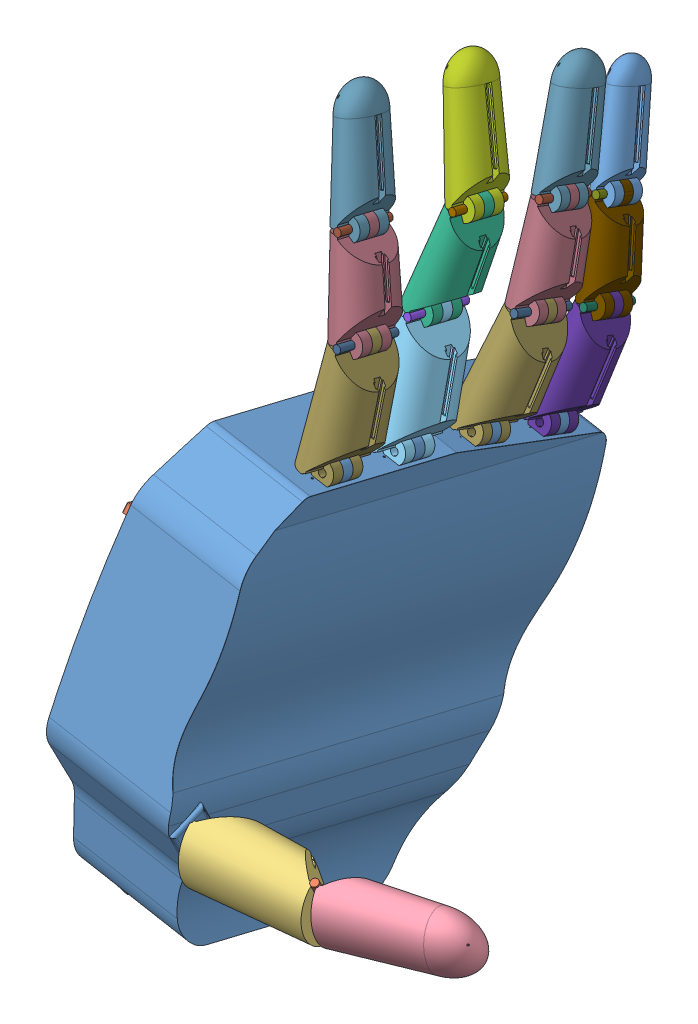
SolidWorks assembly hand_ass_v2, configuration Default. Lengths in mm.
Overall size (122.49 222.13 158.08).
29 component instances, 20 part files, 48 mates.
Components (placement in the parent):
- mainbody_v2-4: mainbody_v2 [Default] at (1393.0939 256.2845 230.0733) x (-0.03967 -0.262646 -0.964076) z (0.98509 -0.171926 0.006304) size (116.82 115 48.77)
- Mate1t-4: Mate1t [Default] at (1443.7902 225.3063 267.9284) x (0.146425 0.857082 0.493933) z (0.670742 0.280983 -0.686407) size (23 2 2)
- Part1t-3: Part1t [Default] at (1431.2867 235.9478 276.4521) x (0.146425 0.857082 0.493933) z (-0.086451 0.508491 -0.856716) size (80.14 37 28.83)
- Part2t-3: Part2t [Default] at (1462.1105 235.1801 268.6506) x (0.146425 0.857082 0.493933) z (-0.264208 0.51506 -0.815419) size (22.13 38.57 15.06)
- Part1m-2: Part1m [Default] at (1414.4402 322.5973 216.192) x (-0.03967 -0.262646 -0.964076) z (0.999177 -0.002227 -0.040508) size (67.14 37 33.3)
- Part2m-2: Part2m [Default] at (1416.9612 349.6562 208.7166) x (-0.03967 -0.262646 -0.964076) z (0.980971 -0.193758 0.012421) size (18.99 32 13.25)
- Part3m-2: Part3m [Default] at (1414.6092 375.7736 201.6979) x (-0.03967 -0.262646 -0.964076) z (0.948609 0.293255 -0.118926) size (16.1 35.5 11.04)
- Mate1-2: Mate1 [Default] at (1415.2589 339.0559 221.0098) x (-0.03967 -0.262646 -0.964076) z (0.870094 0.465305 -0.162567) size (18 2 2)
- Mate2-2: Mate2 [Default] at (1420.1608 363.3694 213.1471) x (-0.03967 -0.262646 -0.964076) z (0.88018 0.447523 -0.158138) size (16 2 2)
- Mate1i-7: Mate1i [Default] at (1419.1567 328.7029 194.6213) x (-0.061096 -0.383846 -0.921374) z (0.853883 0.457912 -0.247388) size (18 2 2)
- Mate2i-7: Mate2i [Default] at (1415.3779 344.2512 169.9444) x (0.061096 0.383846 0.921374) z (-0.994886 0.097798 0.025228) size (16 2 2)
- Part1i-6: Part1i [Default] at (1415.7923 312.9467 191.6404) x (-0.061096 -0.383846 -0.921374) z (0.98509 -0.171926 0.006304) size (67.02 35 36.64)
- Part2-6: Part2 [Default] at (1416.6054 336.7334 181.6776) x (-0.061096 -0.383846 -0.921374) z (0.991581 0.082247 -0.100016) size (18.98 30 13.22)
- Part3i-6: Part3i [Default] at (1412.8163 360.7728 171.9137) x (-0.061096 -0.383846 -0.921374) z (0.980311 0.150581 -0.127736) size (16.1 33.51 11.04)
- Mate1p-2: Mate1p [Default] at (1417.5601 318.7755 173.3582) x (-0.061096 -0.383846 -0.921374) z (0.991721 -0.127797 -0.01252) size (16 2 2)
- Mate2p-2: Mate2p [Default] at (1411.96 339.126 164.166) x (-0.061096 -0.383846 -0.921374) z (0.997555 0.007899 -0.069439) size (14 2 2)
- Part1p-2: Part1p [Default] at (1414.4302 303.698 171.1644) x (-0.061096 -0.383846 -0.921374) z (0.98509 -0.171926 0.006304) size (18.99 34 13.27)
- Part2p-2: Part2p [Default] at (1413.7865 326.3018 161.7901) x (-0.061096 -0.383846 -0.921374) z (0.968644 0.199919 -0.147517) size (16.86 29 11.21)
- Part3p-2: Part3p [Default] at (1408.3506 348.6966 152.8208) x (-0.061096 -0.383846 -0.921374) z (0.974142 0.178236 -0.138849) size (14.11 31.5 9.04)
- Mate1i-8: Mate1i [Default] at (1416.3045 338.1976 225.4891) x (0.03967 0.262646 0.964076) z (-0.987081 -0.139593 0.078646) size (18 2 2)
- Mate2i-8: Mate2i [Default] at (1409.7839 360.8016 220.6372) x (0.03967 0.262646 0.964076) z (-0.919513 -0.368003 0.138092) size (16 2 2)
- Part1i-7: Part1i [Default] at (1415.7465 327.3903 237.7916) x (-0.03967 -0.262646 -0.964076) z (0.998985 -0.031014 -0.032657) size (67.02 35 36.64)
- Part3i-7: Part3i [Default] at (1405.8994 376.6502 224.7772) x (-0.03967 -0.262646 -0.964076) z (0.963202 0.246636 -0.106826) size (16.1 33.51 11.04)
- Part2-7: Part2 [Default] at (1412.6818 352.0877 231.19) x (-0.03967 -0.262646 -0.964076) z (0.961097 0.253914 -0.108722) size (18.98 30 13.22)
- SERVO 2-2: SERVO 2 [Default] at (1375.2699 258.4985 245.0042) x (0.374746 0.816954 0.438351) z (0.900147 -0.433837 0.039007) size (32 28.96 12.1)
- SERVO 2-3: SERVO 2 [Default] at (1399.6817 275.2259 280.8947) x (-0.970737 0.2395 0.017575) z (-0.100414 -0.338334 -0.935653) size (32 28.96 12.1)
- SERVO 2-4: SERVO 2 [Default] at (1411.5824 241.8867 212.5876) x (0.093781 0.315033 0.944436) z (-0.990432 0.125987 0.056324) size (32 28.96 12.1)
- SERVO 2-6: SERVO 2 [Default] at (1414.0198 249.6937 180.1774) x (0.274408 0.279911 0.919973) z (-0.954781 0.193152 0.226022) size (32 28.96 12.1)
- SERVO 2-7: SERVO 2 [Default] at (1409.5967 265.7988 229.5325) x (0.0903 0.334214 0.938161) z (-0.97905 0.202412 0.022128) size (32 28.96 12.1)
Mates (geometry in assembly coordinates):
- Concentric1: concentric anti-aligned: cylinder of mainbody_v2-4 through (1415.9837 312.2001 240.3647) axis (0.03967 0.262646 0.964076) radius 1; cylinder of Part1i-7 through (1416.4652 315.3881 252.0667) axis (-0.03967 -0.262646 -0.964076) radius 1
- Coincident1: coincident anti-aligned: plane of mainbody_v2-4 through (1415.9837 312.2001 240.3647) normal (-0.03967 -0.262646 -0.964076); plane of Part1i-7 through (1415.9837 312.2001 240.3647) normal (0.03967 0.262646 0.964076)
- Concentric4: concentric aligned: cylinder of Part1i-7 through (1417.0836 343.3556 244.4221) axis (-0.03967 -0.262646 -0.964076) radius 1; cylinder of Part2-7 through (1417.0387 343.0583 243.331) axis (-0.03967 -0.262646 -0.964076) radius 1
- Coincident4: coincident anti-aligned: plane of Part1i-7 through (1416.6021 340.1676 232.72) normal (-0.03967 -0.262646 -0.964076); plane of Part2-7 through (1416.6021 340.1676 232.72) normal (0.03967 0.262646 0.964076)
- Concentric5: concentric aligned: cylinder of Mate1i-8 through (1417.0186 342.9252 242.8424) axis (-0.03967 -0.262646 -0.964076) radius 1; cylinder of Part2-7 through (1417.0387 343.0583 243.331) axis (-0.03967 -0.262646 -0.964076) radius 1
- Coincident5: coincident anti-aligned: plane of Mate1i-8 through (1416.6616 340.5614 234.1658) normal (0.03967 0.262646 0.964076); plane of Part1i-7 through (1415.7465 327.3903 237.7916) normal (-0.03967 -0.262646 -0.964076)
- Concentric6: concentric anti-aligned: cylinder of Part3i-7 through (1409.8037 360.9329 221.1191) axis (0.03967 0.262646 0.964076) radius 1; cylinder of Part2-7 through (1410.4784 365.3995 237.5145) axis (-0.03967 -0.262646 -0.964076) radius 1
- Coincident6: coincident anti-aligned: plane of Part3i-7 through (1410.0417 362.5088 226.9035) normal (0.03967 0.262646 0.964076); plane of Part2-7 through (1410.0417 362.5088 226.9035) normal (-0.03967 -0.262646 -0.964076)
- Concentric8: concentric anti-aligned: cylinder of Mate2i-8 through (1410.4186 365.004 236.0624) axis (-0.03967 -0.262646 -0.964076) radius 1; cylinder of Part3i-7 through (1409.8037 360.9329 221.1191) axis (0.03967 0.262646 0.964076) radius 1
- Coincident8: coincident anti-aligned: plane of Mate2i-8 through (1410.1012 362.9028 228.3498) normal (0.03967 0.262646 0.964076); plane of Part2-7 through (1412.6818 352.0877 231.19) normal (-0.03967 -0.262646 -0.964076)
- Concentric9: concentric anti-aligned: cylinder of mainbody_v2-4 through (1415.1056 306.3865 219.0249) axis (0.03967 0.262646 0.964076) radius 1; cylinder of Part1m-2 through (1415.5873 309.5752 230.7296) axis (-0.03967 -0.262646 -0.964076) radius 1
- Coincident9: coincident anti-aligned: plane of mainbody_v2-4 through (1415.1056 306.3865 219.0249) normal (-0.03967 -0.262646 -0.964076); plane of Part1m-2 through (1415.1056 306.3865 219.0249) normal (0.03967 0.262646 0.964076)
- Concentric10: concentric aligned: cylinder of Part1m-2 through (1415.324 339.4868 222.5916) axis (-0.03967 -0.262646 -0.964076) radius 1; cylinder of Part2m-2 through (1415.2792 339.1899 221.5017) axis (-0.03967 -0.262646 -0.964076) radius 1
- Coincident10: coincident anti-aligned: plane of Part1m-2 through (1414.8424 336.2981 210.8869) normal (-0.03967 -0.262646 -0.964076); plane of Part2m-2 through (1414.8424 336.2981 210.8869) normal (0.03967 0.262646 0.964076)
- Concentric11: concentric anti-aligned: cylinder of Part2m-2 through (1415.2792 339.1899 221.5017) axis (-0.03967 -0.262646 -0.964076) radius 1; cylinder of Mate1-2 through (1414.5449 334.3282 203.6564) axis (0.03967 0.262646 0.964076) radius 1
- Coincident12: coincident aligned: plane of Part1m-2 through (1414.4402 322.5973 216.192) normal (-0.03967 -0.262646 -0.964076); plane of Mate1-2 through (1414.9019 336.6921 212.3331) normal (-0.03967 -0.262646 -0.964076)
- Concentric12: concentric anti-aligned: cylinder of Part2m-2 through (1420.2207 363.7661 214.603) axis (-0.03967 -0.262646 -0.964076) radius 1; cylinder of Part3m-2 through (1419.5459 359.2984 198.2037) axis (0.03967 0.262646 0.964076) radius 1
- Coincident13: coincident anti-aligned: plane of Part2m-2 through (1419.7839 360.8743 203.9882) normal (-0.03967 -0.262646 -0.964076); plane of Part3m-2 through (1419.7839 360.8743 203.9882) normal (0.03967 0.262646 0.964076)
- Concentric13: concentric aligned: cylinder of Part3m-2 through (1419.5459 359.2984 198.2037) axis (0.03967 0.262646 0.964076) radius 1; cylinder of Mate2-2 through (1419.5261 359.1671 197.7219) axis (0.03967 0.262646 0.964076) radius 1
- Coincident14: coincident aligned: plane of Part2m-2 through (1416.9612 349.6562 208.7166) normal (-0.03967 -0.262646 -0.964076); plane of Mate2-2 through (1419.8435 361.2683 205.4345) normal (-0.03967 -0.262646 -0.964076)
- Parallel2: parallel anti-aligned: plane of mainbody_v2-4 through (1383.8165 307.0595 209.2378) normal (0.160828 0.907251 -0.388627); plane of Part1i-6 through (1414.6286 303.2312 206.6189) normal (-0.160828 -0.907251 0.388627)
- Concentric14: concentric aligned: cylinder of mainbody_v2-4 through (1414.0344 299.5139 198.9816) axis (-0.061096 -0.383846 -0.921374) radius 1; cylinder of Part1i-6 through (1414.5927 303.0215 207.4011) axis (-0.061096 -0.383846 -0.921374) radius 1
- Coincident17: coincident anti-aligned: plane of mainbody_v2-4 through (1413.8511 298.3624 196.2174) normal (-0.061096 -0.383846 -0.921374); plane of Part1i-6 through (1413.8511 298.3624 196.2174) normal (0.061096 0.383846 0.921374)
- Concentric15: concentric aligned: cylinder of Part1i-6 through (1419.2568 329.3318 196.131) axis (-0.061096 -0.383846 -0.921374) radius 1; cylinder of Part2-6 through (1419.1876 328.8974 195.0882) axis (-0.061096 -0.383846 -0.921374) radius 1
- Coincident18: coincident anti-aligned: plane of Part1i-6 through (1418.6985 325.8242 187.7114) normal (0.061096 0.383846 0.921374); plane of Part2-6 through (1418.6985 325.8242 187.7114) normal (-0.061096 -0.383846 -0.921374)
- Concentric16: concentric anti-aligned: cylinder of Mate1i-7 through (1418.0569 321.7936 178.0366) axis (0.061096 0.383846 0.921374) radius 1; cylinder of Part2-6 through (1419.1876 328.8974 195.0882) axis (-0.061096 -0.383846 -0.921374) radius 1
- Coincident20: coincident aligned: plane of Mate1i-7 through (1418.6068 325.2483 186.329) normal (-0.061096 -0.383846 -0.921374); plane of Part1i-6 through (1415.7923 312.9467 191.6404) normal (-0.061096 -0.383846 -0.921374)
- Concentric17: concentric anti-aligned: cylinder of Part2-6 through (1416.4475 350.9708 186.0741) axis (-0.061096 -0.383846 -0.921374) radius 1; cylinder of Part3i-6 through (1415.4085 344.443 170.4049) axis (0.061096 0.383846 0.921374) radius 1
- Coincident21: coincident anti-aligned: plane of Part2-6 through (1415.9583 347.8976 178.6973) normal (0.061096 0.383846 0.921374); plane of Part3i-6 through (1415.9583 347.8976 178.6973) normal (-0.061096 -0.383846 -0.921374)
- Concentric18: concentric anti-aligned: cylinder of Mate2i-7 through (1416.3555 350.3927 184.6864) axis (-0.061096 -0.383846 -0.921374) radius 1; cylinder of Part3i-6 through (1415.4085 344.443 170.4049) axis (0.061096 0.383846 0.921374) radius 1
- Coincident22: coincident anti-aligned: plane of Mate2i-7 through (1415.8667 347.3219 177.3154) normal (0.061096 0.383846 0.921374); plane of Part2-6 through (1416.6054 336.7334 181.6776) normal (-0.061096 -0.383846 -0.921374)
- Parallel3: parallel anti-aligned: plane of mainbody_v2-4 through (1383.8165 307.0595 209.2378) normal (0.160828 0.907251 -0.388627); plane of Part1p-2 through (1413.1864 294.2119 184.9666) normal (-0.160828 -0.907251 0.388627)
- Concentric19: concentric aligned: cylinder of mainbody_v2-4 through (1412.6598 290.8774 178.2507) axis (-0.061096 -0.383846 -0.921374) radius 1; cylinder of Part1p-2 through (1413.1494 293.9534 185.6343) axis (-0.061096 -0.383846 -0.921374) radius 1
- Coincident24: coincident anti-aligned: plane of mainbody_v2-4 through (1412.4765 289.7259 175.4865) normal (-0.061096 -0.383846 -0.921374); plane of Part1p-2 through (1412.4765 289.7259 175.4865) normal (0.061096 0.383846 0.921374)
- Concentric20: concentric aligned: cylinder of Part1p-2 through (1417.6526 319.3565 174.7528) axis (-0.061096 -0.383846 -0.921374) radius 1; cylinder of Part2p-2 through (1417.5885 318.954 173.7868) axis (-0.061096 -0.383846 -0.921374) radius 1
- Coincident25: coincident anti-aligned: plane of Part1p-2 through (1416.9797 315.1289 164.605) normal (-0.061096 -0.383846 -0.921374); plane of Part2p-2 through (1416.9797 315.1289 164.605) normal (0.061096 0.383846 0.921374)
- Concentric21: concentric anti-aligned: cylinder of Mate1p-2 through (1416.5826 312.6339 158.6162) axis (0.061096 0.383846 0.921374) radius 1; cylinder of Part2p-2 through (1417.5885 318.954 173.7868) axis (-0.061096 -0.383846 -0.921374) radius 1
- Coincident26: coincident aligned: plane of Mate1p-2 through (1417.0713 315.7047 165.9872) normal (-0.061096 -0.383846 -0.921374); plane of Part1p-2 through (1414.4302 303.698 171.1644) normal (-0.061096 -0.383846 -0.921374)
- Concentric22: concentric anti-aligned: cylinder of Part2p-2 through (1412.0496 339.6884 165.5161) axis (-0.061096 -0.383846 -0.921374) radius 1; cylinder of Part3p-2 through (1411.0742 333.5602 150.806) axis (0.061096 0.383846 0.921374) radius 1
- Coincident27: coincident anti-aligned: plane of Part2p-2 through (1411.4407 335.8633 156.3343) normal (-0.061096 -0.383846 -0.921374); plane of Part3p-2 through (1411.4407 335.8633 156.3343) normal (0.061096 0.383846 0.921374)
- Concentric24: concentric aligned: cylinder of Mate2p-2 through (1411.1047 333.7521 151.2667) axis (0.061096 0.383846 0.921374) radius 1; cylinder of Part3p-2 through (1411.0742 333.5602 150.806) axis (0.061096 0.383846 0.921374) radius 1
- Coincident28: coincident aligned: plane of Mate2p-2 through (1411.5324 336.439 157.7163) normal (-0.061096 -0.383846 -0.921374); plane of Part2p-2 through (1413.7865 326.3018 161.7901) normal (-0.061096 -0.383846 -0.921374)
- Concentric25: concentric anti-aligned: cylinder of mainbody_v2-4 through (1415.1452 239.0135 278.9547) axis (-0.146425 -0.857082 -0.493933) radius 1; cylinder of Part1t-3 through (1413.0554 226.7806 271.9049) axis (0.146425 0.857082 0.493933) radius 1
- Concentric27: concentric anti-aligned: cylinder of Part1t-3 through (1443.6039 224.2155 267.2998) axis (0.146425 0.857082 0.493933) radius 1; cylinder of Part2t-3 through (1446.5723 241.591 277.3132) axis (-0.146425 -0.857082 -0.493933) radius 1
- Coincident30: coincident anti-aligned: plane of mainbody_v2-4 through (1415.1452 239.0135 278.9547) normal (0.146425 0.857082 0.493933); plane of Part1t-3 through (1415.1452 239.0135 278.9547) normal (-0.146425 -0.857082 -0.493933)
- Coincident32: coincident anti-aligned: plane of Part1t-3 through (1445.6938 236.4485 274.3496) normal (0.146425 0.857082 0.493933); plane of Part2t-3 through (1445.6938 236.4485 274.3496) normal (-0.146425 -0.857082 -0.493933)
- Concentric28: concentric aligned: cylinder of Mate1t-4 through (1447.158 245.0192 279.2888) axis (-0.146425 -0.857082 -0.493933) radius 1; cylinder of Part2t-3 through (1446.5723 241.591 277.3132) axis (-0.146425 -0.857082 -0.493933) radius 1
- Coincident33: coincident aligned: plane of Mate1t-4 through (1445.4741 235.1627 273.6086) normal (0.146425 0.857082 0.493933); plane of Part1t-3 through (1431.2867 235.9478 276.4521) normal (0.146425 0.857082 0.493933)
